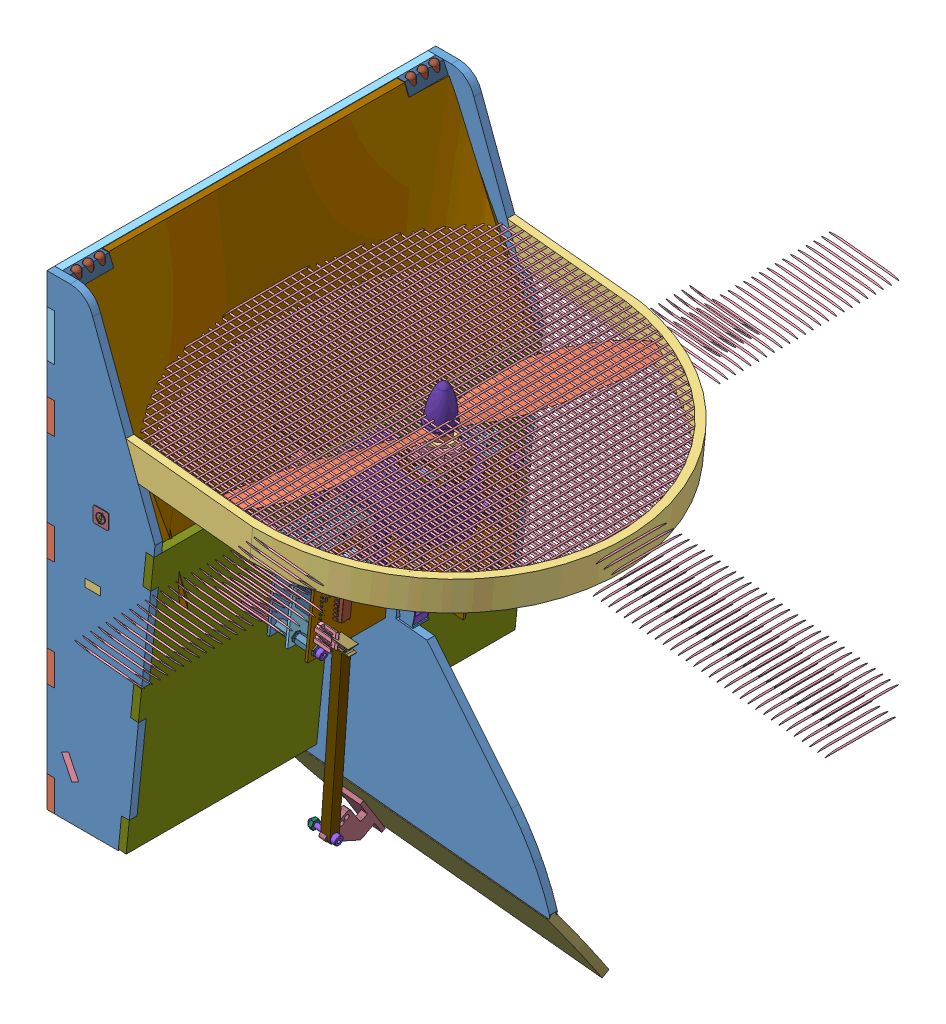
SolidWorks assembly AssTotaleSimu5, configuration Défaut. Lengths in mm. (continued)
Components (placement in the parent): (continued)
- AssStructSimu-1: AssStructSimu [Défaut] at (-125.7658 -1.8483 624.6548) x (1 0 0) z (0 0 -1) size (253.25 324.59 251.6) (continued)
  - AssProtec-1: AssProtec [Défaut] at (86.6746 190.4649 284.6351) x (0 0 -1) z (0.101852 -0.9948 0) size (250 237.46 20) (continued)
    - AssGrillage-2: AssGrillage [Défaut] at (339.6086 -132.5428 241.6839) x (0 0 1) z (-1 0 0) size (2.02 237.05 250) (continued)
      - barreau-208: barreau [Défaut] at (-0.1839 -1.5314 233.7823) x (0.998922 0 0.04641) z (0 1 0) size (1 1 400)
      - barreau-209: barreau [Défaut] at (-0.1839 -1.5314 228.7823) x (0.998922 0 0.04641) z (0 1 0) size (1 1 400)
      - barreau-210: barreau [Défaut] at (-0.1839 -1.5314 223.7823) x (0.998922 0 0.04641) z (0 1 0) size (1 1 400)
      - barreau-211: barreau [Défaut] at (-0.1839 -1.5314 218.7823) x (0.998922 0 0.04641) z (0 1 0) size (1 1 400)
      - barreau-212: barreau [Défaut] at (-0.1839 -1.5314 213.7823) x (0.998922 0 0.04641) z (0 1 0) size (1 1 400)
      - barreau-213: barreau [Défaut] at (-0.1839 -1.5314 208.7823) x (0.998922 0 0.04641) z (0 1 0) size (1 1 400)
      - barreau-214: barreau [Défaut] at (-0.1839 -1.5314 203.7823) x (0.998922 0 0.04641) z (0 1 0) size (1 1 400)
  - AssCarte-1: AssCarte [Défaut] at (38.0121 147.1029 290.772) x (-0.101852 0.9948 0) z (0.9948 0.101852 0) size (66.52 130.57 98.72)
    - carte_onduleur_v3-1: carte_onduleur_v3 [Défaut] at (-131.8199 12.0892 20.7912) size (66.52 130.57 82.34)
      - Layer_1-1: Layer_1 [Défaut] at origin size (60 130 1.61)
      - BTN-1: BTN [Défaut] at (-25.5 7.4 0.803) x (0 -1 0) z (0 0 1) size (6.76 3.64 4.37)
        - Open CASCADE STEP translator 6.8 1.2.1-1: Open CASCADE STEP translator 6.8 1.2.1 [Défaut] at origin size (6.76 3.64 4.37)
          - Body_1-1: Body_1 [Défaut] at (-0.5 -2 0) size (6.76 3.64 4.37)
            - =_[0_1_1_3]-1: =_[0_1_1_3] [Défaut] at origin size (6 3.64 4.37)
            - =_[0_1_1_4]-1: =_[0_1_1_4] [Défaut] at origin size (0.38 1 0.67)
            - =_[0_1_1_5]-1: =_[0_1_1_5] [Défaut] at origin size (0.38 1 0.67)
      - CON_IO1-1: CON_IO1 [Défaut] at (-11.3 12.1 0.803) x (0 -1 0) z (0 0 1) size (13 30 57.5)
        - Open CASCADE STEP translator 6.8 1.3.1-1: Open CASCADE STEP translator 6.8 1.3.1 [Défaut] at origin size (13 30 57.5)
          - Body_1_2-1: Body_1_2 [Défaut] at (-3 -15 8) x (0 -1 0) z (-1 0 0) size (30 57.5 13)
            - 1-1: 1 [Défaut] at origin size (30 50 1.61)
            - 10-1: 10 [Défaut] at (-14.395 31.0465 0.803) x (-1 0 0) z (0 0 1) size (5.59 6.35 1.11)
              - =_[0_1_1_4]-1: =_[0_1_1_4] [Défaut] at origin size (5.59 6.35 1.11)
                - 11-1: 11 [Défaut] at (2 3.3 0) x (-1 0 0) z (0 0 1) size (5.59 6.35 1.11)
                  - =_[0_1_1_3]_2-1: =_[0_1_1_3]_2 [Défaut] at origin size (0.44 0.55 0.36)
                  - =_[0_1_1_4]_2-1: =_[0_1_1_4]_2 [Défaut] at origin size (5.59 4.15 0.36)
                  - =_[0_1_1_5]_2-1: =_[0_1_1_5]_2 [Défaut] at origin size (5.35 6.1 1.1)
                  - =_[0_1_1_6]-1: =_[0_1_1_6] [Défaut] at origin size (0.44 0.55 0.36)
                  - =_[0_1_1_7]-1: =_[0_1_1_7] [Défaut] at origin size (0.44 0.55 0.36)
                  - =_[0_1_1_8]-1: =_[0_1_1_8] [Défaut] at origin size (0.44 0.55 0.36)
            - 13-1: 13 [Défaut] at (-12.62 16.6 -0.803) x (-1 0 0) z (0 0 -1) size (5.59 6.35 1.11)
              - =_[0_1_1_13]-1: =_[0_1_1_13] [Défaut] at origin size (5.59 6.35 1.11)
                - 11-1: 11 [Défaut] at (2 3.3 0) x (-1 0 0) z (0 0 1) size (5.59 6.35 1.11)
                  - =_[0_1_1_3]_2-1: =_[0_1_1_3]_2 [Défaut] at origin size (0.44 0.55 0.36)
                  - =_[0_1_1_4]_2-1: =_[0_1_1_4]_2 [Défaut] at origin size (5.59 4.15 0.36)
                  - =_[0_1_1_5]_2-1: =_[0_1_1_5]_2 [Défaut] at origin size (5.35 6.1 1.1)
                  - =_[0_1_1_6]-1: =_[0_1_1_6] [Défaut] at origin size (0.44 0.55 0.36)
                  - =_[0_1_1_7]-1: =_[0_1_1_7] [Défaut] at origin size (0.44 0.55 0.36)
                  - =_[0_1_1_8]-1: =_[0_1_1_8] [Défaut] at origin size (0.44 0.55 0.36)
            - 16-1: 16 [Défaut] at (-4.2 24.2 0.803) x (-1 0 0) z (0 0 1) size (12.8 0.5 13)
              - =_[0_1_1_15]-1: =_[0_1_1_15] [Défaut] at origin size (12.8 0.5 13)
                - 17-1: 17 [Défaut] at (2.7 0 0) x (1 0 0) z (0 -1 0) size (12.8 13 0.5)
            - 19-1: 19 [Défaut] at (-4.1 6.8 0.803) x (-1 0 0) z (0 0 1) size (12.8 0.5 13)
              - =_[0_1_1_18]-1: =_[0_1_1_18] [Défaut] at origin size (12.8 0.5 13)
                - 17-1: 17 [Défaut] at (2.7 0 0) x (1 0 0) z (0 -1 0) size (12.8 13 0.5)
            - 24-1: 24 [Défaut] at (-8.1 16.5 -0.803) x (0 1 0) z (0 0 -1) size (7.75 5.13 1.17)
              - =_[0_1_1_20]-1: =_[0_1_1_20] [Défaut] at origin size (7.75 5.13 1.17)
                - 20-1: 20 [Défaut] at origin size (7.59 5.13 1.07)
                - 21-1: 21 [Défaut] at (-14.478 0 0) x (-1 0 0) z (0 0 1) size (0.76 5.08 1.17)
                - 22-1: 22 [Défaut] at origin size (0.76 5.08 1.17)
            - 35-1: 35 [Défaut] at (-25.3 25.5 0.803) x (0 -1 0) z (0 0 1) size (6.05 5.2 1.7)
              - =_[0_1_1_25]-1: =_[0_1_1_25] [Défaut] at origin size (6.05 5.2 1.7)
                - 25-1: 25 [Défaut] at origin size (4.3 5.2 1.53)
                - 26-1: 26 [Défaut] at origin size (0.88 0.51 1.06)
                - 27-1: 27 [Défaut] at origin size (0.88 0.51 1.06)
                - 28-1: 28 [Défaut] at origin size (0.88 0.51 1.06)
                - 29-1: 29 [Défaut] at origin size (0.88 0.51 1.06)
                - 30-1: 30 [Défaut] at (11.6 -5.08 0) x (-1 0 0) z (0 0 1) size (0.87 0.51 1.06)
                - 31-1: 31 [Défaut] at (11.6 -2.54 0) x (-1 0 0) z (0 0 1) size (0.87 0.51 1.06)
                - 32-1: 32 [Défaut] at (11.6 0 0) x (-1 0 0) z (0 0 1) size (0.87 0.51 1.06)
                - 33-1: 33 [Défaut] at (11.6 2.54 0) x (-1 0 0) z (0 0 1) size (0.87 0.51 1.06)
            - 40-1: 40 [Défaut] at (-27.6 27.2 0.803) size (2.34 1.04 0.5)
              - =_[0_1_1_36]-1: =_[0_1_1_36] [Défaut] at origin size (2.34 1.04 0.5)
                - 36-1: 36 [Défaut] at origin size (2.29 1.04 0.43)
                - 37-1: 37 [Défaut] at (0.3048 0 0) x (-1 0 0) z (0 0 1) size (0.51 1.02 0.5)
                - 38-1: 38 [Défaut] at origin size (0.51 1.02 0.5)
            - 42-1: 42 [Défaut] at (-22.1 21.6 0.803) x (0 1 0) z (0 0 1) size (2.34 1.04 0.5)
              - =_[0_1_1_36]-1: =_[0_1_1_36] [Défaut] at origin size (2.34 1.04 0.5)
                - 36-1: 36 [Défaut] at origin size (2.29 1.04 0.43)
                - 37-1: 37 [Défaut] at (0.3048 0 0) x (-1 0 0) z (0 0 1) size (0.51 1.02 0.5)
                - 38-1: 38 [Défaut] at origin size (0.51 1.02 0.5)
            - 47-1: 47 [Défaut] at (-14.7664 14.5 -0.803) x (-1 0 0) z (0 0 -1) size (2.34 1.04 0.5)
              - =_[0_1_1_42]-1: =_[0_1_1_42] [Défaut] at origin size (2.34 1.04 0.5)
                - 43-1: 43 [Défaut] at origin size (2.29 1.04 0.43)
                - 44-1: 44 [Défaut] at (0.3048 0 0) x (-1 0 0) z (0 0 1) size (0.51 1.02 0.5)
                - 45-1: 45 [Défaut] at origin size (0.51 1.02 0.5)
            - 57-1: 57 [Défaut] at (-15.3 2.7 -0.803) x (0 -1 0) z (0 0 -1) size (10.36 15.24 6.14)
              - =_[0_1_1_47]-1: =_[0_1_1_47] [Défaut] at origin size (10.36 15.24 6.14)
                - 55-1: 55 [Défaut] at (1.8 -1.2 3) x (1 0 0) z (0 1 0) size (10.36 6.14 15.24)
                  - 54-1: 54 [Défaut] at origin size (10.36 6.14 7.62)
                    - 52-1: 52 [Défaut] at origin size (10.36 6.14 2.54)
                      - 48-1: 48 [Défaut] at origin size (8.4 2.54 2.54)
                      - 49-1: 49 [Défaut] at (-0.0461 1.2682 1.27) x (0 0 -1) z (0.999998 -0.002105 0) size (1.95 5.07 7.58)
                    - 52-2: 52 [Défaut] at (0 0 -2.54) size (10.36 6.14 2.54)
                      - 48-1: 48 [Défaut] at origin size (8.4 2.54 2.54)
                      - 49-1: 49 [Défaut] at (-0.0461 1.2682 1.27) x (0 0 -1) z (0.999998 -0.002105 0) size (1.95 5.07 7.58)
                    - 52-3: 52 [Défaut] at (0 0 -5.08) size (10.36 6.14 2.54)
                      - 48-1: 48 [Défaut] at origin size (8.4 2.54 2.54)
                      - 49-1: 49 [Défaut] at (-0.0461 1.2682 1.27) x (0 0 -1) z (0.999998 -0.002105 0) size (1.95 5.07 7.58)
                  - 54-2: 54 [Défaut] at (0 0 -7.62) size (10.36 6.14 7.62)
                    - 52-1: 52 [Défaut] at origin size (10.36 6.14 2.54)
                      - 48-1: 48 [Défaut] at origin size (8.4 2.54 2.54)
                      - 49-1: 49 [Défaut] at (-0.0461 1.2682 1.27) x (0 0 -1) z (0.999998 -0.002105 0) size (1.95 5.07 7.58)
                    - 52-2: 52 [Défaut] at (0 0 -2.54) size (10.36 6.14 2.54)
                      - 48-1: 48 [Défaut] at origin size (8.4 2.54 2.54)
                      - 49-1: 49 [Défaut] at (-0.0461 1.2682 1.27) x (0 0 -1) z (0.999998 -0.002105 0) size (1.95 5.07 7.58)
                    - 52-3: 52 [Défaut] at (0 0 -5.08) size (10.36 6.14 2.54)
                      - 48-1: 48 [Défaut] at origin size (8.4 2.54 2.54)
                      - 49-1: 49 [Défaut] at (-0.0461 1.2682 1.27) x (0 0 -1) z (0.999998 -0.002105 0) size (1.95 5.07 7.58)
            - 59-1: 59 [Défaut] at (-26.5 31 0.803) x (0 -1 0) z (0 0 1) size (2.34 1.04 0.5)
              - =_[0_1_1_42]-1: =_[0_1_1_42] [Défaut] at origin size (2.34 1.04 0.5)
                - 43-1: 43 [Défaut] at origin size (2.29 1.04 0.43)
                - 44-1: 44 [Défaut] at (0.3048 0 0) x (-1 0 0) z (0 0 1) size (0.51 1.02 0.5)
                - 45-1: 45 [Défaut] at origin size (0.51 1.02 0.5)
            - 61-1: 61 [Défaut] at (-21.6 17.8 0.803) x (-1 0 0) z (0 0 1) size (2.34 1.04 0.5)
              - =_[0_1_1_42]-1: =_[0_1_1_42] [Défaut] at origin size (2.34 1.04 0.5)
                - 43-1: 43 [Défaut] at origin size (2.29 1.04 0.43)
                - 44-1: 44 [Défaut] at (0.3048 0 0) x (-1 0 0) z (0 0 1) size (0.51 1.02 0.5)
                - 45-1: 45 [Défaut] at origin size (0.51 1.02 0.5)
            - 74-1: 74 [Défaut] at (-4.9 41.8 0.803) x (0 -1 0) z (0 0 1) size (6 4.9 1.75)
              - =_[0_1_1_56]-1: =_[0_1_1_56] [Défaut] at origin size (6 4.9 1.75)
                - 72-1: 72 [Défaut] at origin size (6 4.9 1.75)
                  - =_[0_1_1_2]-1: =_[0_1_1_2] [Défaut] at origin size (3.9 4.9 1.57)
                  - =_[0_1_1_3]-1: =_[0_1_1_3] [Défaut] at origin size (6 4.22 1)
                    - =_[0_1_1_60]-1: =_[0_1_1_60] [Défaut] at origin size (1.05 0.41 1)
                    - =_[0_1_1_61]-1: =_[0_1_1_61] [Défaut] at origin size (1.05 0.41 1)
                    - =_[0_1_1_62]-1: =_[0_1_1_62] [Défaut] at origin size (1.05 0.41 1)
                    - =_[0_1_1_63]-1: =_[0_1_1_63] [Défaut] at origin size (1.05 0.41 1)
                    - =_[0_1_1_64]-1: =_[0_1_1_64] [Défaut] at origin size (1.05 0.41 1)
                    - =_[0_1_1_65]-1: =_[0_1_1_65] [Défaut] at origin size (1.05 0.41 1)
                    - =_[0_1_1_66]-1: =_[0_1_1_66] [Défaut] at origin size (1.05 0.41 1)
                    - =_[0_1_1_67]-1: =_[0_1_1_67] [Défaut] at origin size (1.05 0.41 1)
            - 76-1: 76 [Défaut] at (-8.5 40.5664 0.803) x (0 1 0) z (0 0 1) size (2.34 1.04 0.5)
              - =_[0_1_1_42]-1: =_[0_1_1_42] [Défaut] at origin size (2.34 1.04 0.5)
                - 43-1: 43 [Défaut] at origin size (2.29 1.04 0.43)
                - 44-1: 44 [Défaut] at (0.3048 0 0) x (-1 0 0) z (0 0 1) size (0.51 1.02 0.5)
                - 45-1: 45 [Défaut] at origin size (0.51 1.02 0.5)
            - 78-1: 78 [Défaut] at (-5.9 46.4 0.803) x (-1 0 0) z (0 0 1) size (2.34 1.04 0.5)
              - =_[0_1_1_42]-1: =_[0_1_1_42] [Défaut] at origin size (2.34 1.04 0.5)
                - 43-1: 43 [Défaut] at origin size (2.29 1.04 0.43)
                - 44-1: 44 [Défaut] at (0.3048 0 0) x (-1 0 0) z (0 0 1) size (0.51 1.02 0.5)
                - 45-1: 45 [Défaut] at origin size (0.51 1.02 0.5)
            - 80-1: 80 [Défaut] at (-7 48.1 0.803) size (2.34 1.04 0.5)
              - =_[0_1_1_42]-1: =_[0_1_1_42] [Défaut] at origin size (2.34 1.04 0.5)
                - 43-1: 43 [Défaut] at origin size (2.29 1.04 0.43)
                - 44-1: 44 [Défaut] at (0.3048 0 0) x (-1 0 0) z (0 0 1) size (0.51 1.02 0.5)
                - 45-1: 45 [Défaut] at origin size (0.51 1.02 0.5)
            - 82-1: 82 [Défaut] at (-6 37.1 0.803) size (2.34 1.04 0.5)
              - =_[0_1_1_42]-1: =_[0_1_1_42] [Défaut] at origin size (2.34 1.04 0.5)
                - 43-1: 43 [Défaut] at origin size (2.29 1.04 0.43)
                - 44-1: 44 [Défaut] at (0.3048 0 0) x (-1 0 0) z (0 0 1) size (0.51 1.02 0.5)
                - 45-1: 45 [Défaut] at origin size (0.51 1.02 0.5)
      - CON_IO2-1: CON_IO2 [Défaut] at (-11.3 -2.7 0.803) x (0 -1 0) z (0 0 1) size (13 30 57.5)
        - Open CASCADE STEP translator 6.8 1.4.1-1: Open CASCADE STEP translator 6.8 1.4.1 [Défaut] at origin size (13 30 57.5)
          - Body_1_2-1: Body_1_2 [Défaut] at (-3 -15 8) x (0 -1 0) z (-1 0 0) size (30 57.5 13)
            - 1-1: 1 [Défaut] at origin size (30 50 1.61)
            - 10-1: 10 [Défaut] at (-14.395 31.0465 0.803) x (-1 0 0) z (0 0 1) size (5.59 6.35 1.11)
              - =_[0_1_1_4]-1: =_[0_1_1_4] [Défaut] at origin size (5.59 6.35 1.11)
                - 11-1: 11 [Défaut] at (2 3.3 0) x (-1 0 0) z (0 0 1) size (5.59 6.35 1.11)
                  - =_[0_1_1_3]_2-1: =_[0_1_1_3]_2 [Défaut] at origin size (0.44 0.55 0.36)
                  - =_[0_1_1_4]_2-1: =_[0_1_1_4]_2 [Défaut] at origin size (5.59 4.15 0.36)
                  - =_[0_1_1_5]_2-1: =_[0_1_1_5]_2 [Défaut] at origin size (5.35 6.1 1.1)
                  - =_[0_1_1_6]-1: =_[0_1_1_6] [Défaut] at origin size (0.44 0.55 0.36)
                  - =_[0_1_1_7]-1: =_[0_1_1_7] [Défaut] at origin size (0.44 0.55 0.36)
                  - =_[0_1_1_8]-1: =_[0_1_1_8] [Défaut] at origin size (0.44 0.55 0.36)
            - 13-1: 13 [Défaut] at (-12.62 16.6 -0.803) x (-1 0 0) z (0 0 -1) size (5.59 6.35 1.11)
              - =_[0_1_1_13]-1: =_[0_1_1_13] [Défaut] at origin size (5.59 6.35 1.11)
                - 11-1: 11 [Défaut] at (2 3.3 0) x (-1 0 0) z (0 0 1) size (5.59 6.35 1.11)
                  - =_[0_1_1_3]_2-1: =_[0_1_1_3]_2 [Défaut] at origin size (0.44 0.55 0.36)
                  - =_[0_1_1_4]_2-1: =_[0_1_1_4]_2 [Défaut] at origin size (5.59 4.15 0.36)
                  - =_[0_1_1_5]_2-1: =_[0_1_1_5]_2 [Défaut] at origin size (5.35 6.1 1.1)
                  - =_[0_1_1_6]-1: =_[0_1_1_6] [Défaut] at origin size (0.44 0.55 0.36)
                  - =_[0_1_1_7]-1: =_[0_1_1_7] [Défaut] at origin size (0.44 0.55 0.36)
                  - =_[0_1_1_8]-1: =_[0_1_1_8] [Défaut] at origin size (0.44 0.55 0.36)
            - 16-1: 16 [Défaut] at (-4.2 24.2 0.803) x (-1 0 0) z (0 0 1) size (12.8 0.5 13)
              - =_[0_1_1_15]-1: =_[0_1_1_15] [Défaut] at origin size (12.8 0.5 13)
                - 17-1: 17 [Défaut] at (2.7 0 0) x (1 0 0) z (0 -1 0) size (12.8 13 0.5)
            - 19-1: 19 [Défaut] at (-4.1 6.8 0.803) x (-1 0 0) z (0 0 1) size (12.8 0.5 13)
              - =_[0_1_1_18]-1: =_[0_1_1_18] [Défaut] at origin size (12.8 0.5 13)
                - 17-1: 17 [Défaut] at (2.7 0 0) x (1 0 0) z (0 -1 0) size (12.8 13 0.5)
            - 24-1: 24 [Défaut] at (-8.1 16.5 -0.803) x (0 1 0) z (0 0 -1) size (7.75 5.13 1.17)
              - =_[0_1_1_20]-1: =_[0_1_1_20] [Défaut] at origin size (7.75 5.13 1.17)
                - 20-1: 20 [Défaut] at origin size (7.59 5.13 1.07)
                - 21-1: 21 [Défaut] at (-14.478 0 0) x (-1 0 0) z (0 0 1) size (0.76 5.08 1.17)
                - 22-1: 22 [Défaut] at origin size (0.76 5.08 1.17)
            - 35-1: 35 [Défaut] at (-25.3 25.5 0.803) x (0 -1 0) z (0 0 1) size (6.05 5.2 1.7)
              - =_[0_1_1_25]-1: =_[0_1_1_25] [Défaut] at origin size (6.05 5.2 1.7)
                - 25-1: 25 [Défaut] at origin size (4.3 5.2 1.53)
                - 26-1: 26 [Défaut] at origin size (0.88 0.51 1.06)
                - 27-1: 27 [Défaut] at origin size (0.88 0.51 1.06)
                - 28-1: 28 [Défaut] at origin size (0.88 0.51 1.06)
                - 29-1: 29 [Défaut] at origin size (0.88 0.51 1.06)
                - 30-1: 30 [Défaut] at (11.6 -5.08 0) x (-1 0 0) z (0 0 1) size (0.87 0.51 1.06)
                - 31-1: 31 [Défaut] at (11.6 -2.54 0) x (-1 0 0) z (0 0 1) size (0.87 0.51 1.06)
                - 32-1: 32 [Défaut] at (11.6 0 0) x (-1 0 0) z (0 0 1) size (0.87 0.51 1.06)
                - 33-1: 33 [Défaut] at (11.6 2.54 0) x (-1 0 0) z (0 0 1) size (0.87 0.51 1.06)
            - 40-1: 40 [Défaut] at (-27.6 27.2 0.803) size (2.34 1.04 0.5)
              - =_[0_1_1_36]-1: =_[0_1_1_36] [Défaut] at origin size (2.34 1.04 0.5)
                - 36-1: 36 [Défaut] at origin size (2.29 1.04 0.43)
                - 37-1: 37 [Défaut] at (0.3048 0 0) x (-1 0 0) z (0 0 1) size (0.51 1.02 0.5)
                - 38-1: 38 [Défaut] at origin size (0.51 1.02 0.5)
            - 42-1: 42 [Défaut] at (-22.1 21.6 0.803) x (0 1 0) z (0 0 1) size (2.34 1.04 0.5)
              - =_[0_1_1_36]-1: =_[0_1_1_36] [Défaut] at origin size (2.34 1.04 0.5)
                - 36-1: 36 [Défaut] at origin size (2.29 1.04 0.43)
                - 37-1: 37 [Défaut] at (0.3048 0 0) x (-1 0 0) z (0 0 1) size (0.51 1.02 0.5)
                - 38-1: 38 [Défaut] at origin size (0.51 1.02 0.5)
            - 47-1: 47 [Défaut] at (-14.7664 14.5 -0.803) x (-1 0 0) z (0 0 -1) size (2.34 1.04 0.5)
              - =_[0_1_1_42]-1: =_[0_1_1_42] [Défaut] at origin size (2.34 1.04 0.5)
                - 43-1: 43 [Défaut] at origin size (2.29 1.04 0.43)
                - 44-1: 44 [Défaut] at (0.3048 0 0) x (-1 0 0) z (0 0 1) size (0.51 1.02 0.5)
                - 45-1: 45 [Défaut] at origin size (0.51 1.02 0.5)
            - 57-1: 57 [Défaut] at (-15.3 2.7 -0.803) x (0 -1 0) z (0 0 -1) size (10.36 15.24 6.14)
              - =_[0_1_1_47]-1: =_[0_1_1_47] [Défaut] at origin size (10.36 15.24 6.14)
                - 55-1: 55 [Défaut] at (1.8 -1.2 3) x (1 0 0) z (0 1 0) size (10.36 6.14 15.24)
                  - 54-1: 54 [Défaut] at origin size (10.36 6.14 7.62)
                    - 52-1: 52 [Défaut] at origin size (10.36 6.14 2.54)
                      - 48-1: 48 [Défaut] at origin size (8.4 2.54 2.54)
                      - 49-1: 49 [Défaut] at (-0.0461 1.2682 1.27) x (0 0 -1) z (0.999998 -0.002105 0) size (1.95 5.07 7.58)
                    - 52-2: 52 [Défaut] at (0 0 -2.54) size (10.36 6.14 2.54)
                      - 48-1: 48 [Défaut] at origin size (8.4 2.54 2.54)
                      - 49-1: 49 [Défaut] at (-0.0461 1.2682 1.27) x (0 0 -1) z (0.999998 -0.002105 0) size (1.95 5.07 7.58)
                    - 52-3: 52 [Défaut] at (0 0 -5.08) size (10.36 6.14 2.54)
                      - 48-1: 48 [Défaut] at origin size (8.4 2.54 2.54)
                      - 49-1: 49 [Défaut] at (-0.0461 1.2682 1.27) x (0 0 -1) z (0.999998 -0.002105 0) size (1.95 5.07 7.58)
                  - 54-2: 54 [Défaut] at (0 0 -7.62) size (10.36 6.14 7.62)
                    - 52-1: 52 [Défaut] at origin size (10.36 6.14 2.54)
                      - 48-1: 48 [Défaut] at origin size (8.4 2.54 2.54)
                      - 49-1: 49 [Défaut] at (-0.0461 1.2682 1.27) x (0 0 -1) z (0.999998 -0.002105 0) size (1.95 5.07 7.58)
                    - 52-2: 52 [Défaut] at (0 0 -2.54) size (10.36 6.14 2.54)
                      - 48-1: 48 [Défaut] at origin size (8.4 2.54 2.54)
                      - 49-1: 49 [Défaut] at (-0.0461 1.2682 1.27) x (0 0 -1) z (0.999998 -0.002105 0) size (1.95 5.07 7.58)
                    - 52-3: 52 [Défaut] at (0 0 -5.08) size (10.36 6.14 2.54)
                      - 48-1: 48 [Défaut] at origin size (8.4 2.54 2.54)
                      - 49-1: 49 [Défaut] at (-0.0461 1.2682 1.27) x (0 0 -1) z (0.999998 -0.002105 0) size (1.95 5.07 7.58)
            - 59-1: 59 [Défaut] at (-26.5 31 0.803) x (0 -1 0) z (0 0 1) size (2.34 1.04 0.5)
              - =_[0_1_1_42]-1: =_[0_1_1_42] [Défaut] at origin size (2.34 1.04 0.5)
                - 43-1: 43 [Défaut] at origin size (2.29 1.04 0.43)
                - 44-1: 44 [Défaut] at (0.3048 0 0) x (-1 0 0) z (0 0 1) size (0.51 1.02 0.5)
                - 45-1: 45 [Défaut] at origin size (0.51 1.02 0.5)
            - 61-1: 61 [Défaut] at (-21.6 17.8 0.803) x (-1 0 0) z (0 0 1) size (2.34 1.04 0.5)
              - =_[0_1_1_42]-1: =_[0_1_1_42] [Défaut] at origin size (2.34 1.04 0.5)
                - 43-1: 43 [Défaut] at origin size (2.29 1.04 0.43)
                - 44-1: 44 [Défaut] at (0.3048 0 0) x (-1 0 0) z (0 0 1) size (0.51 1.02 0.5)
                - 45-1: 45 [Défaut] at origin size (0.51 1.02 0.5)
            - 74-1: 74 [Défaut] at (-4.9 41.8 0.803) x (0 -1 0) z (0 0 1) size (6 4.9 1.75)
              - =_[0_1_1_56]-1: =_[0_1_1_56] [Défaut] at origin size (6 4.9 1.75)
                - 72-1: 72 [Défaut] at origin size (6 4.9 1.75)
                  - =_[0_1_1_2]-1: =_[0_1_1_2] [Défaut] at origin size (3.9 4.9 1.57)
                  - =_[0_1_1_3]-1: =_[0_1_1_3] [Défaut] at origin size (6 4.22 1)
                    - =_[0_1_1_60]-1: =_[0_1_1_60] [Défaut] at origin size (1.05 0.41 1)
                    - =_[0_1_1_61]-1: =_[0_1_1_61] [Défaut] at origin size (1.05 0.41 1)
                    - =_[0_1_1_62]-1: =_[0_1_1_62] [Défaut] at origin size (1.05 0.41 1)
                    - =_[0_1_1_63]-1: =_[0_1_1_63] [Défaut] at origin size (1.05 0.41 1)
                    - =_[0_1_1_64]-1: =_[0_1_1_64] [Défaut] at origin size (1.05 0.41 1)
                    - =_[0_1_1_65]-1: =_[0_1_1_65] [Défaut] at origin size (1.05 0.41 1)
                    - =_[0_1_1_66]-1: =_[0_1_1_66] [Défaut] at origin size (1.05 0.41 1)
                    - =_[0_1_1_67]-1: =_[0_1_1_67] [Défaut] at origin size (1.05 0.41 1)
            - 76-1: 76 [Défaut] at (-8.5 40.5664 0.803) x (0 1 0) z (0 0 1) size (2.34 1.04 0.5)
              - =_[0_1_1_42]-1: =_[0_1_1_42] [Défaut] at origin size (2.34 1.04 0.5)
                - 43-1: 43 [Défaut] at origin size (2.29 1.04 0.43)
                - 44-1: 44 [Défaut] at (0.3048 0 0) x (-1 0 0) z (0 0 1) size (0.51 1.02 0.5)
                - 45-1: 45 [Défaut] at origin size (0.51 1.02 0.5)
            - 78-1: 78 [Défaut] at (-5.9 46.4 0.803) x (-1 0 0) z (0 0 1) size (2.34 1.04 0.5)
              - =_[0_1_1_42]-1: =_[0_1_1_42] [Défaut] at origin size (2.34 1.04 0.5)
                - 43-1: 43 [Défaut] at origin size (2.29 1.04 0.43)
                - 44-1: 44 [Défaut] at (0.3048 0 0) x (-1 0 0) z (0 0 1) size (0.51 1.02 0.5)
                - 45-1: 45 [Défaut] at origin size (0.51 1.02 0.5)
            - 80-1: 80 [Défaut] at (-7 48.1 0.803) size (2.34 1.04 0.5)
              - =_[0_1_1_42]-1: =_[0_1_1_42] [Défaut] at origin size (2.34 1.04 0.5)
                - 43-1: 43 [Défaut] at origin size (2.29 1.04 0.43)
                - 44-1: 44 [Défaut] at (0.3048 0 0) x (-1 0 0) z (0 0 1) size (0.51 1.02 0.5)
                - 45-1: 45 [Défaut] at origin size (0.51 1.02 0.5)
            - 82-1: 82 [Défaut] at (-6 37.1 0.803) size (2.34 1.04 0.5)
              - =_[0_1_1_42]-1: =_[0_1_1_42] [Défaut] at origin size (2.34 1.04 0.5)
                - 43-1: 43 [Défaut] at origin size (2.29 1.04 0.43)
                - 44-1: 44 [Défaut] at (0.3048 0 0) x (-1 0 0) z (0 0 1) size (0.51 1.02 0.5)
                - 45-1: 45 [Défaut] at origin size (0.51 1.02 0.5)
      - CON_IO3-1: CON_IO3 [Défaut] at (-11.3 -17.7 0.803) x (0 -1 0) z (0 0 1) size (13 30 57.5)
        - Open CASCADE STEP translator 6.8 1.5.1-1: Open CASCADE STEP translator 6.8 1.5.1 [Défaut] at origin size (13 30 57.5)
          - Body_1_2-1: Body_1_2 [Défaut] at (-3 -15 8) x (0 -1 0) z (-1 0 0) size (30 57.5 13)
            - 1-1: 1 [Défaut] at origin size (30 50 1.61)
            - 10-1: 10 [Défaut] at (-14.395 31.0465 0.803) x (-1 0 0) z (0 0 1) size (5.59 6.35 1.11)
              - =_[0_1_1_4]-1: =_[0_1_1_4] [Défaut] at origin size (5.59 6.35 1.11)
                - 11-1: 11 [Défaut] at (2 3.3 0) x (-1 0 0) z (0 0 1) size (5.59 6.35 1.11)
                  - =_[0_1_1_3]_2-1: =_[0_1_1_3]_2 [Défaut] at origin size (0.44 0.55 0.36)
                  - =_[0_1_1_4]_2-1: =_[0_1_1_4]_2 [Défaut] at origin size (5.59 4.15 0.36)
                  - =_[0_1_1_5]_2-1: =_[0_1_1_5]_2 [Défaut] at origin size (5.35 6.1 1.1)
                  - =_[0_1_1_6]-1: =_[0_1_1_6] [Défaut] at origin size (0.44 0.55 0.36)
                  - =_[0_1_1_7]-1: =_[0_1_1_7] [Défaut] at origin size (0.44 0.55 0.36)
                  - =_[0_1_1_8]-1: =_[0_1_1_8] [Défaut] at origin size (0.44 0.55 0.36)
            - 13-1: 13 [Défaut] at (-12.62 16.6 -0.803) x (-1 0 0) z (0 0 -1) size (5.59 6.35 1.11)
              - =_[0_1_1_13]-1: =_[0_1_1_13] [Défaut] at origin size (5.59 6.35 1.11)
                - 11-1: 11 [Défaut] at (2 3.3 0) x (-1 0 0) z (0 0 1) size (5.59 6.35 1.11)
                  - =_[0_1_1_3]_2-1: =_[0_1_1_3]_2 [Défaut] at origin size (0.44 0.55 0.36)
                  - =_[0_1_1_4]_2-1: =_[0_1_1_4]_2 [Défaut] at origin size (5.59 4.15 0.36)
                  - =_[0_1_1_5]_2-1: =_[0_1_1_5]_2 [Défaut] at origin size (5.35 6.1 1.1)
                  - =_[0_1_1_6]-1: =_[0_1_1_6] [Défaut] at origin size (0.44 0.55 0.36)
                  - =_[0_1_1_7]-1: =_[0_1_1_7] [Défaut] at origin size (0.44 0.55 0.36)
                  - =_[0_1_1_8]-1: =_[0_1_1_8] [Défaut] at origin size (0.44 0.55 0.36)
            - 16-1: 16 [Défaut] at (-4.2 24.2 0.803) x (-1 0 0) z (0 0 1) size (12.8 0.5 13)
              - =_[0_1_1_15]-1: =_[0_1_1_15] [Défaut] at origin size (12.8 0.5 13)
                - 17-1: 17 [Défaut] at (2.7 0 0) x (1 0 0) z (0 -1 0) size (12.8 13 0.5)
            - 19-1: 19 [Défaut] at (-4.1 6.8 0.803) x (-1 0 0) z (0 0 1) size (12.8 0.5 13)
              - =_[0_1_1_18]-1: =_[0_1_1_18] [Défaut] at origin size (12.8 0.5 13)
                - 17-1: 17 [Défaut] at (2.7 0 0) x (1 0 0) z (0 -1 0) size (12.8 13 0.5)
            - 24-1: 24 [Défaut] at (-8.1 16.5 -0.803) x (0 1 0) z (0 0 -1) size (7.75 5.13 1.17)
              - =_[0_1_1_20]-1: =_[0_1_1_20] [Défaut] at origin size (7.75 5.13 1.17)
                - 20-1: 20 [Défaut] at origin size (7.59 5.13 1.07)
                - 21-1: 21 [Défaut] at (-14.478 0 0) x (-1 0 0) z (0 0 1) size (0.76 5.08 1.17)
                - 22-1: 22 [Défaut] at origin size (0.76 5.08 1.17)
            - 35-1: 35 [Défaut] at (-25.3 25.5 0.803) x (0 -1 0) z (0 0 1) size (6.05 5.2 1.7)
              - =_[0_1_1_25]-1: =_[0_1_1_25] [Défaut] at origin size (6.05 5.2 1.7)
                - 25-1: 25 [Défaut] at origin size (4.3 5.2 1.53)
                - 26-1: 26 [Défaut] at origin size (0.88 0.51 1.06)
                - 27-1: 27 [Défaut] at origin size (0.88 0.51 1.06)
                - 28-1: 28 [Défaut] at origin size (0.88 0.51 1.06)
                - 29-1: 29 [Défaut] at origin size (0.88 0.51 1.06)
                - 30-1: 30 [Défaut] at (11.6 -5.08 0) x (-1 0 0) z (0 0 1) size (0.87 0.51 1.06)
                - 31-1: 31 [Défaut] at (11.6 -2.54 0) x (-1 0 0) z (0 0 1) size (0.87 0.51 1.06)
                - 32-1: 32 [Défaut] at (11.6 0 0) x (-1 0 0) z (0 0 1) size (0.87 0.51 1.06)
                - 33-1: 33 [Défaut] at (11.6 2.54 0) x (-1 0 0) z (0 0 1) size (0.87 0.51 1.06)
            - 40-1: 40 [Défaut] at (-27.6 27.2 0.803) size (2.34 1.04 0.5)
              - =_[0_1_1_36]-1: =_[0_1_1_36] [Défaut] at origin size (2.34 1.04 0.5)
                - 36-1: 36 [Défaut] at origin size (2.29 1.04 0.43)
                - 37-1: 37 [Défaut] at (0.3048 0 0) x (-1 0 0) z (0 0 1) size (0.51 1.02 0.5)
                - 38-1: 38 [Défaut] at origin size (0.51 1.02 0.5)
            - 42-1: 42 [Défaut] at (-22.1 21.6 0.803) x (0 1 0) z (0 0 1) size (2.34 1.04 0.5)
              - =_[0_1_1_36]-1: =_[0_1_1_36] [Défaut] at origin size (2.34 1.04 0.5)
                - 36-1: 36 [Défaut] at origin size (2.29 1.04 0.43)
                - 37-1: 37 [Défaut] at (0.3048 0 0) x (-1 0 0) z (0 0 1) size (0.51 1.02 0.5)
                - 38-1: 38 [Défaut] at origin size (0.51 1.02 0.5)
            - 47-1: 47 [Défaut] at (-14.7664 14.5 -0.803) x (-1 0 0) z (0 0 -1) size (2.34 1.04 0.5)
              - =_[0_1_1_42]-1: =_[0_1_1_42] [Défaut] at origin size (2.34 1.04 0.5)
                - 43-1: 43 [Défaut] at origin size (2.29 1.04 0.43)
                - 44-1: 44 [Défaut] at (0.3048 0 0) x (-1 0 0) z (0 0 1) size (0.51 1.02 0.5)
                - 45-1: 45 [Défaut] at origin size (0.51 1.02 0.5)
            - 57-1: 57 [Défaut] at (-15.3 2.7 -0.803) x (0 -1 0) z (0 0 -1) size (10.36 15.24 6.14)
              - =_[0_1_1_47]-1: =_[0_1_1_47] [Défaut] at origin size (10.36 15.24 6.14)
                - 55-1: 55 [Défaut] at (1.8 -1.2 3) x (1 0 0) z (0 1 0) size (10.36 6.14 15.24)
                  - 54-1: 54 [Défaut] at origin size (10.36 6.14 7.62)
                    - 52-1: 52 [Défaut] at origin size (10.36 6.14 2.54)
                      - 48-1: 48 [Défaut] at origin size (8.4 2.54 2.54)
                      - 49-1: 49 [Défaut] at (-0.0461 1.2682 1.27) x (0 0 -1) z (0.999998 -0.002105 0) size (1.95 5.07 7.58)
                    - 52-2: 52 [Défaut] at (0 0 -2.54) size (10.36 6.14 2.54)
                      - 48-1: 48 [Défaut] at origin size (8.4 2.54 2.54)
                      - 49-1: 49 [Défaut] at (-0.0461 1.2682 1.27) x (0 0 -1) z (0.999998 -0.002105 0) size (1.95 5.07 7.58)
                    - 52-3: 52 [Défaut] at (0 0 -5.08) size (10.36 6.14 2.54)
                      - 48-1: 48 [Défaut] at origin size (8.4 2.54 2.54)
                      - 49-1: 49 [Défaut] at (-0.0461 1.2682 1.27) x (0 0 -1) z (0.999998 -0.002105 0) size (1.95 5.07 7.58)
                  - 54-2: 54 [Défaut] at (0 0 -7.62) size (10.36 6.14 7.62)
                    - 52-1: 52 [Défaut] at origin size (10.36 6.14 2.54)
                      - 48-1: 48 [Défaut] at origin size (8.4 2.54 2.54)
                      - 49-1: 49 [Défaut] at (-0.0461 1.2682 1.27) x (0 0 -1) z (0.999998 -0.002105 0) size (1.95 5.07 7.58)
                    - 52-2: 52 [Défaut] at (0 0 -2.54) size (10.36 6.14 2.54)
                      - 48-1: 48 [Défaut] at origin size (8.4 2.54 2.54)
                      - 49-1: 49 [Défaut] at (-0.0461 1.2682 1.27) x (0 0 -1) z (0.999998 -0.002105 0) size (1.95 5.07 7.58)
                    - 52-3: 52 [Défaut] at (0 0 -5.08) size (10.36 6.14 2.54)
                      - 48-1: 48 [Défaut] at origin size (8.4 2.54 2.54)
                      - 49-1: 49 [Défaut] at (-0.0461 1.2682 1.27) x (0 0 -1) z (0.999998 -0.002105 0) size (1.95 5.07 7.58)
            - 59-1: 59 [Défaut] at (-26.5 31 0.803) x (0 -1 0) z (0 0 1) size (2.34 1.04 0.5)
              - =_[0_1_1_42]-1: =_[0_1_1_42] [Défaut] at origin size (2.34 1.04 0.5)
                - 43-1: 43 [Défaut] at origin size (2.29 1.04 0.43)
                - 44-1: 44 [Défaut] at (0.3048 0 0) x (-1 0 0) z (0 0 1) size (0.51 1.02 0.5)
                - 45-1: 45 [Défaut] at origin size (0.51 1.02 0.5)
            - 61-1: 61 [Défaut] at (-21.6 17.8 0.803) x (-1 0 0) z (0 0 1) size (2.34 1.04 0.5)
              - =_[0_1_1_42]-1: =_[0_1_1_42] [Défaut] at origin size (2.34 1.04 0.5)
                - 43-1: 43 [Défaut] at origin size (2.29 1.04 0.43)
                - 44-1: 44 [Défaut] at (0.3048 0 0) x (-1 0 0) z (0 0 1) size (0.51 1.02 0.5)
                - 45-1: 45 [Défaut] at origin size (0.51 1.02 0.5)
            - 74-1: 74 [Défaut] at (-4.9 41.8 0.803) x (0 -1 0) z (0 0 1) size (6 4.9 1.75)
              - =_[0_1_1_56]-1: =_[0_1_1_56] [Défaut] at origin size (6 4.9 1.75)
                - 72-1: 72 [Défaut] at origin size (6 4.9 1.75)
                  - =_[0_1_1_2]-1: =_[0_1_1_2] [Défaut] at origin size (3.9 4.9 1.57)
                  - =_[0_1_1_3]-1: =_[0_1_1_3] [Défaut] at origin size (6 4.22 1)
                    - =_[0_1_1_60]-1: =_[0_1_1_60] [Défaut] at origin size (1.05 0.41 1)
                    - =_[0_1_1_61]-1: =_[0_1_1_61] [Défaut] at origin size (1.05 0.41 1)
                    - =_[0_1_1_62]-1: =_[0_1_1_62] [Défaut] at origin size (1.05 0.41 1)
                    - =_[0_1_1_63]-1: =_[0_1_1_63] [Défaut] at origin size (1.05 0.41 1)
                    - =_[0_1_1_64]-1: =_[0_1_1_64] [Défaut] at origin size (1.05 0.41 1)
                    - =_[0_1_1_65]-1: =_[0_1_1_65] [Défaut] at origin size (1.05 0.41 1)
                    - =_[0_1_1_66]-1: =_[0_1_1_66] [Défaut] at origin size (1.05 0.41 1)
                    - =_[0_1_1_67]-1: =_[0_1_1_67] [Défaut] at origin size (1.05 0.41 1)
            - 76-1: 76 [Défaut] at (-8.5 40.5664 0.803) x (0 1 0) z (0 0 1) size (2.34 1.04 0.5)
              - =_[0_1_1_42]-1: =_[0_1_1_42] [Défaut] at origin size (2.34 1.04 0.5)
                - 43-1: 43 [Défaut] at origin size (2.29 1.04 0.43)
                - 44-1: 44 [Défaut] at (0.3048 0 0) x (-1 0 0) z (0 0 1) size (0.51 1.02 0.5)
                - 45-1: 45 [Défaut] at origin size (0.51 1.02 0.5)
            - 78-1: 78 [Défaut] at (-5.9 46.4 0.803) x (-1 0 0) z (0 0 1) size (2.34 1.04 0.5)
              - =_[0_1_1_42]-1: =_[0_1_1_42] [Défaut] at origin size (2.34 1.04 0.5)
                - 43-1: 43 [Défaut] at origin size (2.29 1.04 0.43)
                - 44-1: 44 [Défaut] at (0.3048 0 0) x (-1 0 0) z (0 0 1) size (0.51 1.02 0.5)
                - 45-1: 45 [Défaut] at origin size (0.51 1.02 0.5)
            - 80-1: 80 [Défaut] at (-7 48.1 0.803) size (2.34 1.04 0.5)
              - =_[0_1_1_42]-1: =_[0_1_1_42] [Défaut] at origin size (2.34 1.04 0.5)
                - 43-1: 43 [Défaut] at origin size (2.29 1.04 0.43)
                - 44-1: 44 [Défaut] at (0.3048 0 0) x (-1 0 0) z (0 0 1) size (0.51 1.02 0.5)
                - 45-1: 45 [Défaut] at origin size (0.51 1.02 0.5)
            - 82-1: 82 [Défaut] at (-6 37.1 0.803) size (2.34 1.04 0.5)
              - =_[0_1_1_42]-1: =_[0_1_1_42] [Défaut] at origin size (2.34 1.04 0.5)
                - 43-1: 43 [Défaut] at origin size (2.29 1.04 0.43)
                - 44-1: 44 [Défaut] at (0.3048 0 0) x (-1 0 0) z (0 0 1) size (0.51 1.02 0.5)
                - 45-1: 45 [Défaut] at origin size (0.51 1.02 0.5)
      - C1_1-1: C1_1 [Défaut] at (-20.6336 6.4 -0.803) x (1 0 0) z (0 0 -1) size (2.34 1.04 0.5)
        - Open CASCADE STEP translator 6.8 1.6.1-1: Open CASCADE STEP translator 6.8 1.6.1 [Défaut] at origin size (2.34 1.04 0.5)
          - Body_1-1: Body_1 [Défaut] at origin size (2.29 1.04 0.43)
          - Pin_1-1: Pin_1 [Défaut] at (0.3048 0 0) x (-1 0 0) z (0 0 1) size (0.51 1.02 0.5)
          - Pin_2-1: Pin_2 [Défaut] at origin size (0.51 1.02 0.5)
      - C1_2-1: C1_2 [Défaut] at (-24.2 6.4 -0.803) x (1 0 0) z (0 0 -1) size (2.34 1.04 0.5)
        - Open CASCADE STEP translator 6.8 1.6.1-1: Open CASCADE STEP translator 6.8 1.6.1 [Défaut] at origin size (2.34 1.04 0.5)
          - Body_1-1: Body_1 [Défaut] at origin size (2.29 1.04 0.43)
          - Pin_1-1: Pin_1 [Défaut] at (0.3048 0 0) x (-1 0 0) z (0 0 1) size (0.51 1.02 0.5)
          - Pin_2-1: Pin_2 [Défaut] at origin size (0.51 1.02 0.5)
      - C_F-1: C_F [Défaut] at (-16.2432 4.45 -0.803) x (0 -1 0) z (0 0 -1) size (2.34 1.04 0.5)
        - Open CASCADE STEP translator 6.8 1.6.1-1: Open CASCADE STEP translator 6.8 1.6.1 [Défaut] at origin size (2.34 1.04 0.5)
          - Body_1-1: Body_1 [Défaut] at origin size (2.29 1.04 0.43)
          - Pin_1-1: Pin_1 [Défaut] at (0.3048 0 0) x (-1 0 0) z (0 0 1) size (0.51 1.02 0.5)
          - Pin_2-1: Pin_2 [Défaut] at origin size (0.51 1.02 0.5)
      - D_LED_STATE1-1: D_LED_STATE1 [Défaut] at (-6.8906 -21.6 0.803) size (2.34 1.04 0.5)
        - Open CASCADE STEP translator 6.8 1.6.1-1: Open CASCADE STEP translator 6.8 1.6.1 [Défaut] at origin size (2.34 1.04 0.5)
          - Body_1-1: Body_1 [Défaut] at origin size (2.29 1.04 0.43)
          - Pin_1-1: Pin_1 [Défaut] at (0.3048 0 0) x (-1 0 0) z (0 0 1) size (0.51 1.02 0.5)
          - Pin_2-1: Pin_2 [Défaut] at origin size (0.51 1.02 0.5)
      - PICKIT-1: PICKIT [Défaut] at (-24.1 -30.5 0.803) size (15.24 5 14.3)
        - Open CASCADE STEP translator 6.8 1.10.1-1: Open CASCADE STEP translator 6.8 1.10.1 [Défaut] at origin size (15.24 5 14.3)
          - Body_1_2-1: Body_1_2 [Défaut] at (6.3 0 12) size (15.24 5 14.3)
      - C_DEC_CUR-1: C_DEC_CUR [Défaut] at (-8.9496 5.7572 -0.803) x (0 1 0) z (0 0 -1) size (2.34 1.04 0.5)
        - Open CASCADE STEP translator 6.8 1.6.1-1: Open CASCADE STEP translator 6.8 1.6.1 [Défaut] at origin size (2.34 1.04 0.5)
          - Body_1-1: Body_1 [Défaut] at origin size (2.29 1.04 0.43)
          - Pin_1-1: Pin_1 [Défaut] at (0.3048 0 0) x (-1 0 0) z (0 0 1) size (0.51 1.02 0.5)
          - Pin_2-1: Pin_2 [Défaut] at origin size (0.51 1.02 0.5)
      - R_F-1: R_F [Défaut] at (-14.65 4.4432 -0.803) x (0 -1 0) z (0 0 -1) size (2.34 1.04 0.5)
        - Open CASCADE STEP translator 6.8 1.12.1-1: Open CASCADE STEP translator 6.8 1.12.1 [Défaut] at origin size (2.34 1.04 0.5)
          - Body_1_3-1: Body_1_3 [Défaut] at origin size (2.29 1.04 0.43)
          - Pin_1_2-1: Pin_1_2 [Défaut] at (0.3048 0 0) x (-1 0 0) z (0 0 1) size (0.51 1.02 0.5)
          - Pin_2_2-1: Pin_2_2 [Défaut] at origin size (0.51 1.02 0.5)
      - R_GAIN1-1: R_GAIN1 [Défaut] at (-13.95 5.7568 -0.803) x (0 1 0) z (0 0 -1) size (2.34 1.04 0.5)
        - Open CASCADE STEP translator 6.8 1.12.1-1: Open CASCADE STEP translator 6.8 1.12.1 [Défaut] at origin size (2.34 1.04 0.5)
          - Body_1_3-1: Body_1_3 [Défaut] at origin size (2.29 1.04 0.43)
          - Pin_1_2-1: Pin_1_2 [Défaut] at (0.3048 0 0) x (-1 0 0) z (0 0 1) size (0.51 1.02 0.5)
          - Pin_2_2-1: Pin_2_2 [Défaut] at origin size (0.51 1.02 0.5)
      - R_GAIN2-1: R_GAIN2 [Défaut] at (-15.65 7.9176 -0.803) x (0 -1 0) z (0 0 -1) size (2.34 1.04 0.5)
        - Open CASCADE STEP translator 6.8 1.12.1-1: Open CASCADE STEP translator 6.8 1.12.1 [Défaut] at origin size (2.34 1.04 0.5)
          - Body_1_3-1: Body_1_3 [Défaut] at origin size (2.29 1.04 0.43)
          - Pin_1_2-1: Pin_1_2 [Défaut] at (0.3048 0 0) x (-1 0 0) z (0 0 1) size (0.51 1.02 0.5)
          - Pin_2_2-1: Pin_2_2 [Défaut] at origin size (0.51 1.02 0.5)
      - R_LED_STATE1-1: R_LED_STATE1 [Défaut] at (-6.9242 -19.9 0.803) size (2.34 1.04 0.5)
        - Open CASCADE STEP translator 6.8 1.12.1-1: Open CASCADE STEP translator 6.8 1.12.1 [Défaut] at origin size (2.34 1.04 0.5)
          - Body_1_3-1: Body_1_3 [Défaut] at origin size (2.29 1.04 0.43)
          - Pin_1_2-1: Pin_1_2 [Défaut] at (0.3048 0 0) x (-1 0 0) z (0 0 1) size (0.51 1.02 0.5)
          - Pin_2_2-1: Pin_2_2 [Défaut] at origin size (0.51 1.02 0.5)
      - R_RESET1-1: R_RESET1 [Défaut] at (-23 7.9 0.803) size (2.34 1.04 0.5)
        - Open CASCADE STEP translator 6.8 1.12.1-1: Open CASCADE STEP translator 6.8 1.12.1 [Défaut] at origin size (2.34 1.04 0.5)
          - Body_1_3-1: Body_1_3 [Défaut] at origin size (2.29 1.04 0.43)
          - Pin_1_2-1: Pin_1_2 [Défaut] at (0.3048 0 0) x (-1 0 0) z (0 0 1) size (0.51 1.02 0.5)
          - Pin_2_2-1: Pin_2_2 [Défaut] at origin size (0.51 1.02 0.5)
